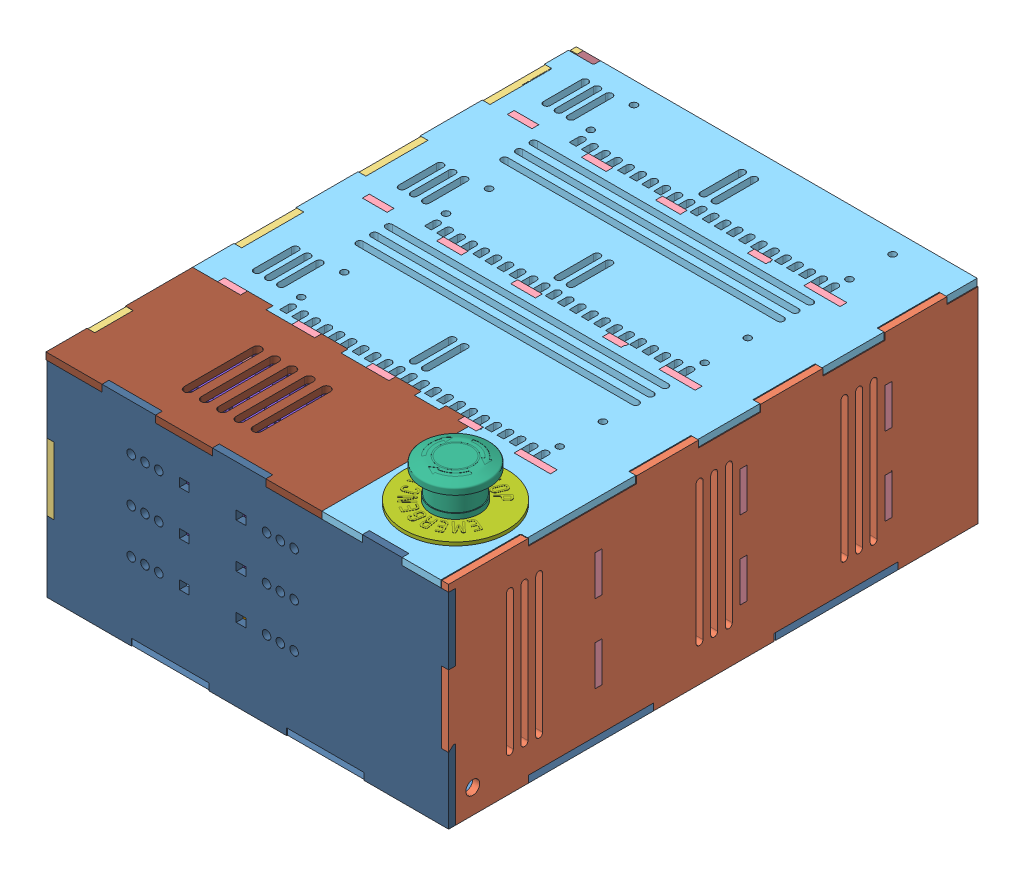
SolidWorks assembly Enclosure Assembly, configuration Default. Lengths in mm.
Overall size (233.5 147.54 307.5).
25 component instances, 14 part files, 42 mates.
Components (placement in the parent):
- Bottom Side-1: Bottom Side [Default] at origin size (233 4 307)
- Right Side-1: Right Side [Default] at (229 4 0.5) size (4 123 307)
- Left Side-1: Left Side [Default] at (0 4 0.4967) size (4 123 307)
- Mid Panel-1: Mid Panel [Default] at (14 119 -84.5) x (1 0 0) z (0 1 0) size (219 4 123)
- Top Side-1: Top Side [Default] at (-0.5 119 0.5) size (233 4 307)
- E Button-1: E Button [Default] at (194.5 123 -42) x (-0.040828 0 0.999166) z (-0.999166 0 -0.040828) size (39 70.54 39)
- E Button Plate-1: E Button Plate [Default] at (194.5 123 -42) x (0.9707 0 0.240295) z (-0.240295 0 0.9707) size (60 2.1 60)
- ODrive-1: ODrive [Default] at (20.1 37.7103 -34.5) x (1 0 0) z (0 1 0) size (147.06 56.62 35.27)
- 50W R47 Power Resistor-1: 50W R47 Power Resistor [Standard] at (58.2633 4 -55.3) size (71 16 29.2)
- 50W R47 Power Resistor-2: 50W R47 Power Resistor [Standard] at (58.2633 4 -32.3) size (71 16 29.2)
- 50W R47 Power Resistor-3: 50W R47 Power Resistor [Standard] at (58.2633 4 -9.3) size (71 16 29.2)
- Front Side-1: Front Side [Default] at (229 119 -3.5) x (-1 0 0) z (0 1 0) size (233 4 123)
- Top Panel-1: Top Panel [Default] at (3.5 119 0.5) size (160 4 89)
- S500 24V Power Supply-2: S500 24V Power Supply [Default] at (229 3.9072 -88.5) x (-1 0 0) z (0 0 -1) size (215 115 50)
- S500 24V Power Supply-3: S500 24V Power Supply [Default] at (229 3.9072 -172.5) x (-1 0 0) z (0 0 -1) size (215 115 50)
- S500 24V Power Supply-4: S500 24V Power Supply [Default] at (229 3.9072 -256.5) x (-1 0 0) z (0 0 -1) size (215 115 50)
- Mid Panel-3: Mid Panel [Default] at (14 119 -168.5) x (1 0 0) z (0 1 0) size (219 4 123)
- Mid Panel-4: Mid Panel [Default] at (14 119 -252.5) x (1 0 0) z (0 1 0) size (219 4 123)
- Back Panel-2: Back Panel [Default] at (31.5 118 -306.5033) x (-1 0 0) z (0 1 0) size (31.5 4 123)
- ODrive-4: ODrive [Default] at (20.1 63.7103 -34.5) x (1 0 0) z (0 1 0) size (147.06 56.62 35.27)
- ODrive-5: ODrive [Default] at (20.1 89.7103 -34.5) x (1 0 0) z (0 1 0) size (147.06 56.62 35.27)
- ODrive Foot-1: ODrive Foot [Default] at (22.0149 24 -84.4335) x (-0.986218 0 -0.165451) z (0.165451 0 -0.986218) size (30 32 19.9)
- ODrive Foot-2: ODrive Foot [Default] at (158.0149 24 -84.4335) x (-0.986218 0 -0.165451) z (0.165451 0 -0.986218) size (30 32 19.9)
- ODrive Foot-3: ODrive Foot [Default] at (22.0149 24 -38.4335) x (-0.986218 0 -0.165451) z (0.165451 0 -0.986218) size (30 32 19.9)
- ODrive Foot-4: ODrive Foot [Default] at (158.0149 24 -38.4335) x (-0.986218 0 -0.165451) z (0.165451 0 -0.986218) size (30 32 19.9)
Mates (geometry in assembly coordinates):
- Coincident1: coincident anti-aligned: plane of Bottom Side-1 through (0 4 0) normal (0 1 0); plane of Right Side-1 through (233 4 0.5) normal (0 -1 0)
- Coincident2: coincident anti-aligned: plane of Bottom Side-1 through (229 0 -307) normal (1 0 0); plane of Right Side-1 through (229 4 0.5) normal (-1 0 0)
- Coincident3: coincident anti-aligned: plane of Bottom Side-1 through (229 0 -45.8333) normal (0 0 1); plane of Right Side-1 through (229 4 -45.8333) normal (0 0 -1)
- Coincident4: coincident anti-aligned: plane of Bottom Side-1 through (0 4 0) normal (0 1 0); plane of Left Side-1 through (4 4 0.4967) normal (0 -1 0)
- Coincident6: coincident aligned: plane of Bottom Side-1 through (0 4 0) normal (-1 0 0); plane of Left Side-1 through (0 4 0.4967) normal (-1 0 0)
- Coincident7: coincident anti-aligned: plane of Bottom Side-1 through (0 0 -45.8333) normal (0 0 1); plane of Left Side-1 through (4 4 -45.8333) normal (0 0 -1)
- Coincident8: coincident anti-aligned: plane of Right Side-1 through (229 4 0.5) normal (-1 0 0); plane of ? through (229 4 -138.5) normal (1 0 0)
- Coincident9: coincident anti-aligned: plane of Bottom Side-1 through (0 4 0) normal (0 1 0); plane of ? through (229 4 -138.5) normal (0 -1 0)
- Coincident10: coincident aligned: plane of Right Side-1 through (233 4 -306.5) normal (0 0 -1); plane of ? through (229 4 -138.5) normal (0 0 -1)
- Coincident11: coincident anti-aligned: plane of Bottom Side-1 through (0 0 -303) normal (0 0 -1); plane of ? through (31.5 5 -303) normal (0 0 1)
- Coincident12: coincident aligned: plane of Bottom Side-1 through (0 0 0) normal (0 -1 0); plane of ? through (4 0 -303) normal (0 -1 0)
- Coincident13: coincident anti-aligned: plane of Left Side-1 through (4 4 0.4967) normal (1 0 0); plane of ? through (4 4 -307) normal (-1 0 0)
- Coincident14: coincident: plane of ? through (229 4 -88.5) normal (0 0 1); plane of Mid Panel-1 through (14 119 -88.5) normal (0 0 -1)
- Coincident15: coincident anti-aligned: plane of Right Side-1 through (229 4 0.5) normal (-1 0 0); plane of Mid Panel-1 through (229 119 -88.5) normal (1 0 0)
- Coincident16: coincident anti-aligned: plane of Bottom Side-1 through (0 4 0) normal (0 1 0); plane of Mid Panel-1 through (14 4 -88.5) normal (0 -1 0)
- Concentric1: concentric anti-aligned: cylinder of Top Side-1 through (194.5 119 -42) axis (0 1 0) radius 11.25; cylinder of E Button-1 through (194.5 110 -42) axis (0 -1 0) radius 10.5
- Coincident20: coincident anti-aligned: plane of Top Side-1 through (-0.5 123 0.5) normal (0 1 0); plane of E Button-1 through (193.9284 123 -28.0117) normal (0 -1 0)
- Concentric2: concentric aligned: cylinder of E Button-1 through (194.5 110 -42) axis (0 -1 0) radius 14; cylinder of E Button Plate-1 through (194.5 125 -42) axis (0 -1 0) radius 11.25
- Coincident21: coincident anti-aligned: plane of Top Side-1 through (-0.5 123 0.5) normal (0 1 0); plane of E Button Plate-1 through (194.5 123 -42) normal (0 -1 0)
- Coincident22: coincident anti-aligned: plane of Mid Panel-1 through (14 119 -84.5) normal (0 0 1); plane of ODrive-1 through (20.1 36 -84.5) normal (0 0 -1)
- Coincident23: coincident aligned: plane of Mid Panel-1 through (14 119 -88.5) normal (-1 0 0); plane of ODrive-1 through (14 48.8903 -49.48) normal (-1 0 0)
- Distance1: distance = 20 mm anti-aligned: plane of ODrive-1 through (20.1 24 -78) normal (0 -1 0); plane of Bottom Side-1 through (0 4 0) normal (0 1 0)
- Coincident25: coincident anti-aligned: plane of Bottom Side-1 through (0 4 0) normal (0 1 0); plane of 50W R47 Power Resistor-1 through (75.1633 4 -55.3) normal (0 -1 0)
- Coincident26: coincident: plane of Mid Panel-1 through (14 119 -84.5) normal (0 0 1); line of 50W R47 Power Resistor-1 through (108.2633 6 -84.5) axis (-1 0 0)
- Coincident28: coincident aligned: plane of Bottom Side-1 through (0 0 0) normal (0 -1 0); plane of Front Side-1 through (4 0 -3.5) normal (0 -1 0)
- Coincident29: coincident aligned: plane of Right Side-1 through (233 4 0.5) normal (0 0 1); plane of Front Side-1 through (229 119 0.5) normal (0 0 1)
- Coincident30: coincident aligned: plane of Left Side-1 through (0 4 0.4967) normal (-1 0 0); plane of Front Side-1 through (0 2 -3.5) normal (-1 0 0)
- Coincident32: coincident aligned: plane of Front Side-1 through (229 119 0.5) normal (0 0 1); plane of Top Panel-1 through (3.5 123 0.5) normal (0 0 1)
- Coincident35: coincident anti-aligned: plane of Mid Panel-1 through (14 119 -88.5) normal (0 0 -1); plane of S500 24V Power Supply-2 through (229 3.9072 -88.5) normal (0 0 1)
- Coincident36: coincident anti-aligned: plane of Right Side-1 through (229 4 0.5) normal (-1 0 0); plane of S500 24V Power Supply-2 through (229 3.9072 -138.5) normal (1 0 0)
- Coincident38: coincident anti-aligned: plane of Mid Panel-1 through (14 119 -88.5) normal (0 1 0); plane of Top Side-1 through (-0.5 119 0.5) normal (0 -1 0)
- Coincident39: coincident anti-aligned: plane of Mid Panel-1 through (14 119 -88.5) normal (0 0 -1); plane of Top Side-1 through (14 119 -88.5) normal (0 0 1)
- Coincident42: coincident anti-aligned: plane of Top Side-1 through (183 119 0.5) normal (1 0 0); plane of Front Side-1 through (183 119 -3.5) normal (-1 0 0)
- Coincident43: coincident aligned: plane of Top Side-1 through (-0.5 123 0.5) normal (0 1 0); plane of Top Panel-1 through (3.5 123 0.5) normal (0 1 0)
- Coincident44: coincident anti-aligned: plane of Top Side-1 through (159.5 119 -84.5) normal (-1 0 0); plane of Top Panel-1 through (159.5 123 0.5) normal (1 0 0)
- Coincident45: coincident anti-aligned: plane of Left Side-1 through (4 79.5 -302.5033) normal (0 0 -1); plane of Back Panel-2 through (31.5 118 -302.5033) normal (0 0 1)
- Coincident47: coincident anti-aligned: plane of Left Side-1 through (4 4 0.4967) normal (1 0 0); plane of Back Panel-2 through (4 119 -302.5033) normal (-1 0 0)
- Distance2: distance = 0.5 mm anti-aligned: plane of Left Side-1 through (4 79.5 -306.5033) normal (0 -1 0); plane of Back Panel-2 through (4 80 -306.5033) normal (0 1 0)
- Coincident49: coincident aligned: plane of Top Side-1 through (-0.5 123 0.5) normal (0 0 1); plane of Top Panel-1 through (3.5 123 0.5) normal (0 0 1)
- Coincident50: coincident anti-aligned: plane of ODrive-1 through (20.1 24 -78) normal (0 -1 0); plane of ODrive Foot-1 through (22.0149 24 -84.4335) normal (0 1 0)
- Coincident51: coincident aligned: plane of ODrive-1 through (23.6495 24 -79.1896) normal (-0.165451 0 0.986218); plane of ODrive Foot-1 through (18.4132 36 -80.068) normal (-0.165451 0 0.986218)
- Coincident52: coincident anti-aligned: plane of ODrive-1 through (20.6908 24 -79.6859) normal (-0.936815 0 0.349824); plane of ODrive Foot-1 through (18.711 36 -84.9877) normal (0.936815 0 -0.349824)
